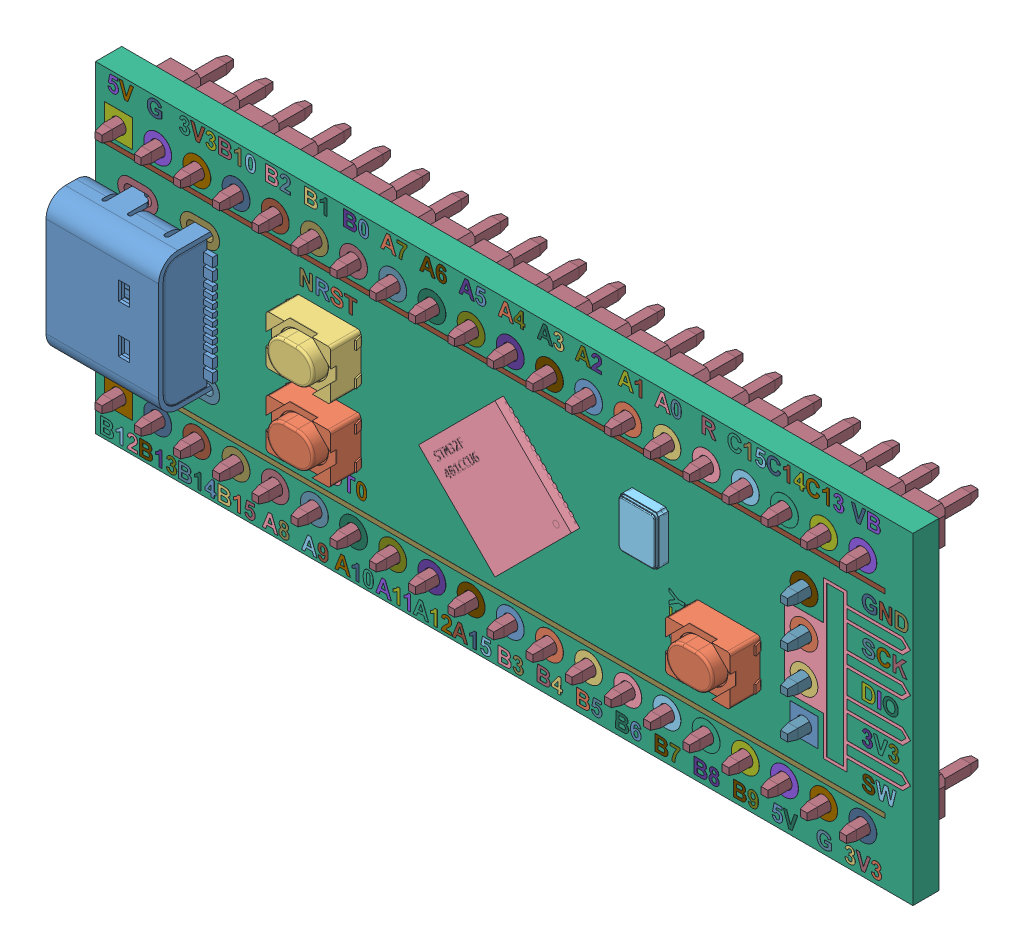
SolidWorks assembly blackpill v2.0 swi, configuration Default. Lengths in mm.
Overall size (53 20.9 10.45).
180 component instances, 176 part files, 0 mates.
Components (placement in the parent):
- blackpill v2.0 swi.STEP-1: blackpill v2.0 swi.STEP [Default] at origin size (53 20.9 10.45)
  - blackpill v2.0.step.STEP-1: blackpill v2.0.step.STEP [Default] at origin size (53 20.9 4.92)
    - USB Type C Port (SMD Type).step.STEP-1: USB Type C Port (SMD Type).step.STEP [Default] at (-19.2 0 3.305) x (0 -1 0) z (0 0 -1) size (8.94 7.9 4.2)
    - PTS810 SJK 250 SMTR LFS--3DModel-STEP-1.step.STEP-1: PTS810 SJK 250 SMTR LFS--3DModel-STEP-1.step.STEP [Default] at (14.5 -1.8498 1.7) x (1 0 0) z (0 -1 0) size (4.6 2.51 3.2)
    - PTS810 SJK 250 SMTR LFS--3DModel-STEP-1.step.STEP-2: PTS810 SJK 250 SMTR LFS--3DModel-STEP-1.step.STEP [Default] at (-11.4 -2.3498 1.7) x (1 0 0) z (0 -1 0) size (4.6 2.51 3.2)
    - PTS810 SJK 250 SMTR LFS--3DModel-STEP-1 v2(Mirror).step.STEP-1: PTS810 SJK 250 SMTR LFS--3DModel-STEP-1 v2(Mirror).step.STEP [Default] at (-11.4 2.3498 1.7) x (1 0 0) z (0 -1 0) size (4.6 2.51 3.2)
    - STM32F411CEU6.step.STEP-1: STM32F411CEU6.step.STEP [Default] at (0 0 1.7) x (-0.707107 -0.707107 0) z (-0.707107 0.707107 0) size (7 0.6 7)
    - ECS-135.60-12-33Q-JES-TR.step.STEP-1: ECS-135.60-12-33Q-JES-TR.step.STEP [Default] at (9.3867 2.3215 1.7) x (0 -1 0) z (-1 0 0) size (3.2 0.8 2.5)
    - DIY_black_pill.step.STEP-1: DIY_black_pill.step.STEP [Default] at origin size (53 20.9 1.7)
    - DIY_black_pill-0.step.STEP-1: DIY_black_pill-0.step.STEP [Default] at origin size (1.8 1.8 1.72)
    - DIY_black_pill-1.step.STEP-1: DIY_black_pill-1.step.STEP [Default] at origin size (1.8 1.8 1.72)
    - DIY_black_pill-2.step.STEP-1: DIY_black_pill-2.step.STEP [Default] at origin size (1.8 1.8 1.72)
    - DIY_black_pill-3.step.STEP-1: DIY_black_pill-3.step.STEP [Default] at origin size (1.8 1.8 1.72)
    - DIY_black_pill-4.step.STEP-1: DIY_black_pill-4.step.STEP [Default] at origin size (1.8 1.8 1.72)
    - DIY_black_pill-5.step.STEP-1: DIY_black_pill-5.step.STEP [Default] at origin size (1.8 1.8 1.72)
    - DIY_black_pill-6.step.STEP-1: DIY_black_pill-6.step.STEP [Default] at origin size (1.8 1.8 1.72)
    - DIY_black_pill-7.step.STEP-1: DIY_black_pill-7.step.STEP [Default] at origin size (1.8 1.8 1.72)
    - DIY_black_pill-8.step.STEP-1: DIY_black_pill-8.step.STEP [Default] at origin size (1.8 1.8 1.72)
    - DIY_black_pill-9.step.STEP-1: DIY_black_pill-9.step.STEP [Default] at origin size (1.8 1.8 1.72)
    - DIY_black_pill-10.step.STEP-1: DIY_black_pill-10.step.STEP [Default] at origin size (1.8 1.8 1.72)
    - DIY_black_pill-11.step.STEP-1: DIY_black_pill-11.step.STEP [Default] at origin size (1.8 1.8 1.72)
    - DIY_black_pill-12.step.STEP-1: DIY_black_pill-12.step.STEP [Default] at origin size (1.8 1.8 1.72)
    - DIY_black_pill-13.step.STEP-1: DIY_black_pill-13.step.STEP [Default] at origin size (1.8 1.8 1.72)
    - DIY_black_pill-14.step.STEP-1: DIY_black_pill-14.step.STEP [Default] at origin size (1.8 1.8 1.72)
    - DIY_black_pill-15.step.STEP-1: DIY_black_pill-15.step.STEP [Default] at origin size (1.8 1.8 1.72)
    - DIY_black_pill-16.step.STEP-1: DIY_black_pill-16.step.STEP [Default] at origin size (1.8 1.8 1.72)
    - DIY_black_pill-17.step.STEP-1: DIY_black_pill-17.step.STEP [Default] at origin size (1.8 1.8 1.72)
    - DIY_black_pill-18.step.STEP-1: DIY_black_pill-18.step.STEP [Default] at origin size (1.8 1.8 1.72)
    - DIY_black_pill-19.step.STEP-1: DIY_black_pill-19.step.STEP [Default] at origin size (1.8 1.8 1.72)
    - DIY_black_pill-20.step.STEP-1: DIY_black_pill-20.step.STEP [Default] at origin size (1.8 1.8 1.72)
    - DIY_black_pill-21.step.STEP-1: DIY_black_pill-21.step.STEP [Default] at origin size (1.8 1.8 1.72)
    - DIY_black_pill-22.step.STEP-1: DIY_black_pill-22.step.STEP [Default] at origin size (1.8 1.8 1.72)
    - DIY_black_pill-23.step.STEP-1: DIY_black_pill-23.step.STEP [Default] at origin size (1.8 1.8 1.72)
    - DIY_black_pill-24.step.STEP-1: DIY_black_pill-24.step.STEP [Default] at origin size (1.8 1.8 1.72)
    - DIY_black_pill-25.step.STEP-1: DIY_black_pill-25.step.STEP [Default] at origin size (1.8 1.8 1.72)
    - DIY_black_pill-26.step.STEP-1: DIY_black_pill-26.step.STEP [Default] at origin size (1.8 1.8 1.72)
    - DIY_black_pill-27.step.STEP-1: DIY_black_pill-27.step.STEP [Default] at origin size (1.8 1.8 1.72)
    - DIY_black_pill-28.step.STEP-1: DIY_black_pill-28.step.STEP [Default] at origin size (1.8 1.8 1.72)
    - DIY_black_pill-29.step.STEP-1: DIY_black_pill-29.step.STEP [Default] at origin size (1.8 1.8 1.72)
    - DIY_black_pill-30.step.STEP-1: DIY_black_pill-30.step.STEP [Default] at origin size (1.8 1.8 1.72)
    - DIY_black_pill-31.step.STEP-1: DIY_black_pill-31.step.STEP [Default] at origin size (1.8 1.8 1.72)
    - DIY_black_pill-32.step.STEP-1: DIY_black_pill-32.step.STEP [Default] at origin size (1.8 1.8 1.72)
    - DIY_black_pill-33.step.STEP-1: DIY_black_pill-33.step.STEP [Default] at origin size (1.8 1.8 1.72)
    - DIY_black_pill-34.step.STEP-1: DIY_black_pill-34.step.STEP [Default] at origin size (1.8 1.8 1.72)
    - DIY_black_pill-35.step.STEP-1: DIY_black_pill-35.step.STEP [Default] at origin size (1.8 1.8 1.72)
    - DIY_black_pill-36.step.STEP-1: DIY_black_pill-36.step.STEP [Default] at origin size (1.8 1.8 1.72)
    - DIY_black_pill-37.step.STEP-1: DIY_black_pill-37.step.STEP [Default] at origin size (1.8 1.8 1.72)
    - DIY_black_pill-38.step.STEP-1: DIY_black_pill-38.step.STEP [Default] at origin size (1.8 1.8 1.72)
    - DIY_black_pill-39.step.STEP-1: DIY_black_pill-39.step.STEP [Default] at origin size (1.8 1.8 1.72)
    - DIY_black_pill-40.step.STEP-1: DIY_black_pill-40.step.STEP [Default] at origin size (51.2 0.3 0.01)
    - DIY_black_pill-41.step.STEP-1: DIY_black_pill-41.step.STEP [Default] at origin size (51.2 0.3 0.01)
    - DIY_black_pill-42.step.STEP-1: DIY_black_pill-42.step.STEP [Default] at origin size (0.93 1 0.01)
    - DIY_black_pill-43.step.STEP-1: DIY_black_pill-43.step.STEP [Default] at origin size (0.94 1.03 0.01)
    - DIY_black_pill-44.step.STEP-1: DIY_black_pill-44.step.STEP [Default] at origin size (0.93 1 0.01)
    - DIY_black_pill-45.step.STEP-1: DIY_black_pill-45.step.STEP [Default] at origin size (0.67 1.02 0.01)
    - DIY_black_pill-46.step.STEP-1: DIY_black_pill-46.step.STEP [Default] at origin size (0.66 1.02 0.01)
    - DIY_black_pill-47.step.STEP-1: DIY_black_pill-47.step.STEP [Default] at origin size (0.84 1 0.01)
    - DIY_black_pill-48.step.STEP-1: DIY_black_pill-48.step.STEP [Default] at origin size (0.67 1.02 0.01)
    - DIY_black_pill-49.step.STEP-1: DIY_black_pill-49.step.STEP [Default] at origin size (0.84 1.01 0.01)
    - DIY_black_pill-50.step.STEP-1: DIY_black_pill-50.step.STEP [Default] at origin size (0.72 1.01 0.01)
    - DIY_black_pill-51.step.STEP-1: DIY_black_pill-51.step.STEP [Default] at origin size (0.84 1 0.01)
    - DIY_black_pill-52.step.STEP-1: DIY_black_pill-52.step.STEP [Default] at origin size (0.67 1 0.01)
    - DIY_black_pill-53.step.STEP-1: DIY_black_pill-53.step.STEP [Default] at origin size (1 1 0.01)
    - DIY_black_pill-54.step.STEP-1: DIY_black_pill-54.step.STEP [Default] at origin size (0.44 1 0.01)
    - DIY_black_pill-55.step.STEP-1: DIY_black_pill-55.step.STEP [Default] at origin size (0.44 1 0.01)
    - DIY_black_pill-56.step.STEP-1: DIY_black_pill-56.step.STEP [Default] at origin size (1 1 0.01)
    - DIY_black_pill-57.step.STEP-1: DIY_black_pill-57.step.STEP [Default] at origin size (0.44 1 0.01)
    - DIY_black_pill-58.step.STEP-1: DIY_black_pill-58.step.STEP [Default] at origin size (0.67 1.02 0.01)
    - DIY_black_pill-59.step.STEP-1: DIY_black_pill-59.step.STEP [Default] at origin size (0.66 1.02 0.01)
    - DIY_black_pill-60.step.STEP-1: DIY_black_pill-60.step.STEP [Default] at origin size (0.67 1 0.01)
    - DIY_black_pill-61.step.STEP-1: DIY_black_pill-61.step.STEP [Default] at origin size (0.84 1 0.01)
    - DIY_black_pill-62.step.STEP-1: DIY_black_pill-62.step.STEP [Default] at origin size (0.44 1 0.01)
    - DIY_black_pill-63.step.STEP-1: DIY_black_pill-63.step.STEP [Default] at origin size (0.66 1.02 0.01)
    - DIY_black_pill-64.step.STEP-1: DIY_black_pill-64.step.STEP [Default] at origin size (0.44 1 0.01)
    - DIY_black_pill-65.step.STEP-1: DIY_black_pill-65.step.STEP [Default] at origin size (0.84 1 0.01)
    - DIY_black_pill-66.step.STEP-1: DIY_black_pill-66.step.STEP [Default] at origin size (0.72 1 0.01)
    - DIY_black_pill-67.step.STEP-1: DIY_black_pill-67.step.STEP [Default] at origin size (0.44 1 0.01)
    - DIY_black_pill-68.step.STEP-1: DIY_black_pill-68.step.STEP [Default] at origin size (0.84 1 0.01)
    - DIY_black_pill-69.step.STEP-1: DIY_black_pill-69.step.STEP [Default] at origin size (1 1 0.01)
    - DIY_black_pill-70.step.STEP-1: DIY_black_pill-70.step.STEP [Default] at origin size (1 1 0.01)
    - DIY_black_pill-71.step.STEP-1: DIY_black_pill-71.step.STEP [Default] at origin size (0.65 1.02 0.01)
    - DIY_black_pill-72.step.STEP-1: DIY_black_pill-72.step.STEP [Default] at origin size (0.44 1 0.01)
    - DIY_black_pill-73.step.STEP-1: DIY_black_pill-73.step.STEP [Default] at origin size (1 1 0.01)
    - DIY_black_pill-74.step.STEP-1: DIY_black_pill-74.step.STEP [Default] at origin size (0.67 1 0.01)
    - DIY_black_pill-75.step.STEP-1: DIY_black_pill-75.step.STEP [Default] at origin size (0.44 1 0.01)
    - DIY_black_pill-76.step.STEP-1: DIY_black_pill-76.step.STEP [Default] at origin size (1 1 0.01)
    - DIY_black_pill-77.step.STEP-1: DIY_black_pill-77.step.STEP [Default] at origin size (0.66 1.02 0.01)
    - DIY_black_pill-78.step.STEP-1: DIY_black_pill-78.step.STEP [Default] at origin size (0.84 1.01 0.01)
    - DIY_black_pill-79.step.STEP-1: DIY_black_pill-79.step.STEP [Default] at origin size (0.67 1.01 0.01)
    - DIY_black_pill-80.step.STEP-1: DIY_black_pill-80.step.STEP [Default] at origin size (0.84 1 0.01)
    - DIY_black_pill-81.step.STEP-1: DIY_black_pill-81.step.STEP [Default] at origin size (0.66 0.99 0.01)
    - DIY_black_pill-82.step.STEP-1: DIY_black_pill-82.step.STEP [Default] at origin size (0.84 1 0.01)
    - DIY_black_pill-83.step.STEP-1: DIY_black_pill-83.step.STEP [Default] at origin size (0.84 1 0.01)
    - DIY_black_pill-84.step.STEP-1: DIY_black_pill-84.step.STEP [Default] at origin size (0.67 1 0.01)
    - DIY_black_pill-85.step.STEP-1: DIY_black_pill-85.step.STEP [Default] at origin size (0.66 1.02 0.01)
    - DIY_black_pill-86.step.STEP-1: DIY_black_pill-86.step.STEP [Default] at origin size (0.66 1.02 0.01)
    - DIY_black_pill-87.step.STEP-1: DIY_black_pill-87.step.STEP [Default] at origin size (0.67 1 0.01)
    - DIY_black_pill-88.step.STEP-1: DIY_black_pill-88.step.STEP [Default] at origin size (0.44 1 0.01)
    - DIY_black_pill-89.step.STEP-1: DIY_black_pill-89.step.STEP [Default] at origin size (0.84 1 0.01)
    - DIY_black_pill-90.step.STEP-1: DIY_black_pill-90.step.STEP [Default] at origin size (1 1 0.01)
    - DIY_black_pill-91.step.STEP-1: DIY_black_pill-91.step.STEP [Default] at origin size (0.84 1 0.01)
    - DIY_black_pill-92.step.STEP-1: DIY_black_pill-92.step.STEP [Default] at origin size (0.44 1 0.01)
    - DIY_black_pill-93.step.STEP-1: DIY_black_pill-93.step.STEP [Default] at origin size (0.87 1.03 0.01)
    - DIY_black_pill-94.step.STEP-1: DIY_black_pill-94.step.STEP [Default] at origin size (0.44 1 0.01)
    - DIY_black_pill-95.step.STEP-1: DIY_black_pill-95.step.STEP [Default] at origin size (0.44 1 0.01)
    - DIY_black_pill-96.step.STEP-1: DIY_black_pill-96.step.STEP [Default] at origin size (0.9 1 0.01)
    - DIY_black_pill-97.step.STEP-1: DIY_black_pill-97.step.STEP [Default] at origin size (0.65 1.02 0.01)
    - DIY_black_pill-98.step.STEP-1: DIY_black_pill-98.step.STEP [Default] at origin size (1 1 0.01)
    - DIY_black_pill-99.step.STEP-1: DIY_black_pill-99.step.STEP [Default] at origin size (0.72 1 0.01)
    - DIY_black_pill-100.step.STEP-1: DIY_black_pill-100.step.STEP [Default] at origin size (1 1 0.01)
    - DIY_black_pill-101.step.STEP-1: DIY_black_pill-101.step.STEP [Default] at origin size (0.67 1.02 0.01)
    - DIY_black_pill-102.step.STEP-1: DIY_black_pill-102.step.STEP [Default] at origin size (0.65 1.02 0.01)
    - DIY_black_pill-103.step.STEP-1: DIY_black_pill-103.step.STEP [Default] at origin size (1 1 0.01)
    - DIY_black_pill-104.step.STEP-1: DIY_black_pill-104.step.STEP [Default] at origin size (0.84 1 0.01)
    - DIY_black_pill-105.step.STEP-1: DIY_black_pill-105.step.STEP [Default] at origin size (0.84 1 0.01)
    - DIY_black_pill-106.step.STEP-1: DIY_black_pill-106.step.STEP [Default] at origin size (0.65 1.02 0.01)
    - DIY_black_pill-107.step.STEP-1: DIY_black_pill-107.step.STEP [Default] at origin size (0.66 1.02 0.01)
    - DIY_black_pill-108.step.STEP-1: DIY_black_pill-108.step.STEP [Default] at origin size (0.66 1.02 0.01)
    - DIY_black_pill-109.step.STEP-1: DIY_black_pill-109.step.STEP [Default] at origin size (0.67 1 0.01)
    - DIY_black_pill-110.step.STEP-1: DIY_black_pill-110.step.STEP [Default] at origin size (0.93 1 0.01)
    - DIY_black_pill-111.step.STEP-1: DIY_black_pill-111.step.STEP [Default] at origin size (0.94 1.03 0.01)
    - DIY_black_pill-112.step.STEP-1: DIY_black_pill-112.step.STEP [Default] at origin size (0.93 1 0.01)
    - DIY_black_pill-113.step.STEP-1: DIY_black_pill-113.step.STEP [Default] at origin size (0.44 1 0.01)
    - DIY_black_pill-114.step.STEP-1: DIY_black_pill-114.step.STEP [Default] at origin size (0.84 1 0.01)
    - DIY_black_pill-115.step.STEP-1: DIY_black_pill-115.step.STEP [Default] at origin size (0.67 1 0.01)
    - DIY_black_pill-116.step.STEP-1: DIY_black_pill-116.step.STEP [Default] at origin size (0.44 1 0.01)
    - DIY_black_pill-117.step.STEP-1: DIY_black_pill-117.step.STEP [Default] at origin size (0.66 0.99 0.01)
    - DIY_black_pill-118.step.STEP-1: DIY_black_pill-118.step.STEP [Default] at origin size (0.84 1 0.01)
    - DIY_black_pill-119.step.STEP-1: DIY_black_pill-119.step.STEP [Default] at origin size (1 1 0.01)
    - DIY_black_pill-120.step.STEP-1: DIY_black_pill-120.step.STEP [Default] at origin size (0.67 1 0.01)
    - DIY_black_pill-121.step.STEP-1: DIY_black_pill-121.step.STEP [Default] at origin size (1 1 0.01)
    - DIY_black_pill-122.step.STEP-1: DIY_black_pill-122.step.STEP [Default] at origin size (0.66 1.02 0.01)
    - DIY_black_pill-123.step.STEP-1: DIY_black_pill-123.step.STEP [Default] at origin size (1 1 0.01)
    - DIY_black_pill-124.step.STEP-1: DIY_black_pill-124.step.STEP [Default] at origin size (0.67 1 0.01)
    - DIY_black_pill-125.step.STEP-1: DIY_black_pill-125.step.STEP [Default] at origin size (0.87 1.03 0.01)
    - DIY_black_pill-126.step.STEP-1: DIY_black_pill-126.step.STEP [Default] at origin size (0.72 1 0.01)
    - DIY_black_pill-127.step.STEP-1: DIY_black_pill-127.step.STEP [Default] at origin size (0.66 1.02 0.01)
    - DIY_black_pill-128.step.STEP-1: DIY_black_pill-128.step.STEP [Default] at origin size (0.87 1.03 0.01)
    - DIY_black_pill-129.step.STEP-1: DIY_black_pill-129.step.STEP [Default] at origin size (0.93 1 0.01)
    - DIY_black_pill-130.step.STEP-1: DIY_black_pill-130.step.STEP [Default] at origin size (0.44 1 0.01)
    - DIY_black_pill-131.step.STEP-1: DIY_black_pill-131.step.STEP [Default] at origin size (2.55 1.5 1.72)
    - DIY_black_pill-132.step.STEP-1: DIY_black_pill-132.step.STEP [Default] at origin size (2.6 1.5 1.72)
    - DIY_black_pill-133.step.STEP-1: DIY_black_pill-133.step.STEP [Default] at origin size (2.55 1.5 1.72)
    - DIY_black_pill-134.step.STEP-1: DIY_black_pill-134.step.STEP [Default] at origin size (2.6 1.5 1.72)
    - DIY_black_pill-135.step.STEP-1: DIY_black_pill-135.step.STEP [Default] at origin size (1 1 0.01)
    - DIY_black_pill-136.step.STEP-1: DIY_black_pill-136.step.STEP [Default] at origin size (0.67 1.01 0.01)
    - DIY_black_pill-137.step.STEP-1: DIY_black_pill-137.step.STEP [Default] at origin size (1.8 1.8 1.72)
    - DIY_black_pill-138.step.STEP-1: DIY_black_pill-138.step.STEP [Default] at origin size (1.8 1.8 1.72)
    - DIY_black_pill-139.step.STEP-1: DIY_black_pill-139.step.STEP [Default] at origin size (1.8 1.8 1.72)
    - DIY_black_pill-140.step.STEP-1: DIY_black_pill-140.step.STEP [Default] at origin size (1.8 1.8 1.72)
    - DIY_black_pill-141.step.STEP-1: DIY_black_pill-141.step.STEP [Default] at origin size (8.17 10.16 0.01)
    - DIY_black_pill-142.step.STEP-1: DIY_black_pill-142.step.STEP [Default] at origin size (1.31 1 0.01)
    - DIY_black_pill-143.step.STEP-1: DIY_black_pill-143.step.STEP [Default] at origin size (0.93 1 0.01)
    - DIY_black_pill-144.step.STEP-1: DIY_black_pill-144.step.STEP [Default] at origin size (0.84 1 0.01)
    - DIY_black_pill-145.step.STEP-1: DIY_black_pill-145.step.STEP [Default] at origin size (0.2 1 0.01)
    - DIY_black_pill-146.step.STEP-1: DIY_black_pill-146.step.STEP [Default] at origin size (0.87 1.03 0.01)
    - DIY_black_pill-147.step.STEP-1: DIY_black_pill-147.step.STEP [Default] at origin size (0.94 1.03 0.01)
    - DIY_black_pill-148.step.STEP-1: DIY_black_pill-148.step.STEP [Default] at origin size (0.79 1 0.01)
    - DIY_black_pill-149.step.STEP-1: DIY_black_pill-149.step.STEP [Default] at origin size (0.84 1 0.01)
    - DIY_black_pill-150.step.STEP-1: DIY_black_pill-150.step.STEP [Default] at origin size (0.9 1 0.01)
    - DIY_black_pill-151.step.STEP-1: DIY_black_pill-151.step.STEP [Default] at origin size (0.81 1.03 0.01)
    - DIY_black_pill-152.step.STEP-1: DIY_black_pill-152.step.STEP [Default] at origin size (0.97 1.03 0.01)
    - DIY_black_pill-153.step.STEP-1: DIY_black_pill-153.step.STEP [Default] at origin size (0.66 1.02 0.01)
    - DIY_black_pill-154.step.STEP-1: DIY_black_pill-154.step.STEP [Default] at origin size (0.66 1.02 0.01)
    - DIY_black_pill-155.step.STEP-1: DIY_black_pill-155.step.STEP [Default] at origin size (0.81 1.03 0.01)
    - DIY_black_pill-156.step.STEP-1: DIY_black_pill-156.step.STEP [Default] at origin size (0.9 1 0.01)
    - DIY_black_pill-157.step.STEP-1: DIY_black_pill-157.step.STEP [Default] at origin size (0.81 1.03 0.01)
    - DIY_black_pill-158.step.STEP-1: DIY_black_pill-158.step.STEP [Default] at origin size (0.97 1.03 0.01)
    - DIY_black_pill-159.step.STEP-1: DIY_black_pill-159.step.STEP [Default] at origin size (0.97 1.03 0.01)
    - DIY_black_pill-160.step.STEP-1: DIY_black_pill-160.step.STEP [Default] at origin size (1.01 0.91 0.01)
    - DIY_black_pill-161.step.STEP-1: DIY_black_pill-161.step.STEP [Default] at origin size (1 0.94 0.01)
    - DIY_black_pill-162.step.STEP-1: DIY_black_pill-162.step.STEP [Default] at origin size (1 0.77 0.01)
    - DIY_black_pill-163.step.STEP-1: DIY_black_pill-163.step.STEP [Default] at origin size (0.79 1 0.01)
    - DIY_black_pill-164.step.STEP-1: DIY_black_pill-164.step.STEP [Default] at origin size (0.65 1.02 0.01)
    - DIY_black_pill-165.step.STEP-1: DIY_black_pill-165.step.STEP [Default] at origin size (0.84 1 0.01)
    - DIY_black_pill-166.step.STEP-1: DIY_black_pill-166.step.STEP [Default] at origin size (0.79 1 0.01)
    - DIY_black_pill-167.step.STEP-1: DIY_black_pill-167.step.STEP [Default] at origin size (0.79 1 0.01)
  - 1x20 Male Pin Header.STEP-1: 1x20 Male Pin Header.STEP [Default] at (23.26 -7.6 0) x (-1 0 0) z (0 -1 0) size (50.8 8.54 2.5)
  - 1x20 Male Pin Header.STEP-2: 1x20 Male Pin Header.STEP [Default] at (23.26 7.6 0) x (-1 0 0) z (0 -1 0) size (50.8 8.54 2.5)
  - 1x4 Male Pin Header.STEP-1: 1x4 Male Pin Header.STEP [Default] at (19.45 -3.81 0) x (0 1 0) z (-1 0 0) size (10.17 8.54 2.5)
